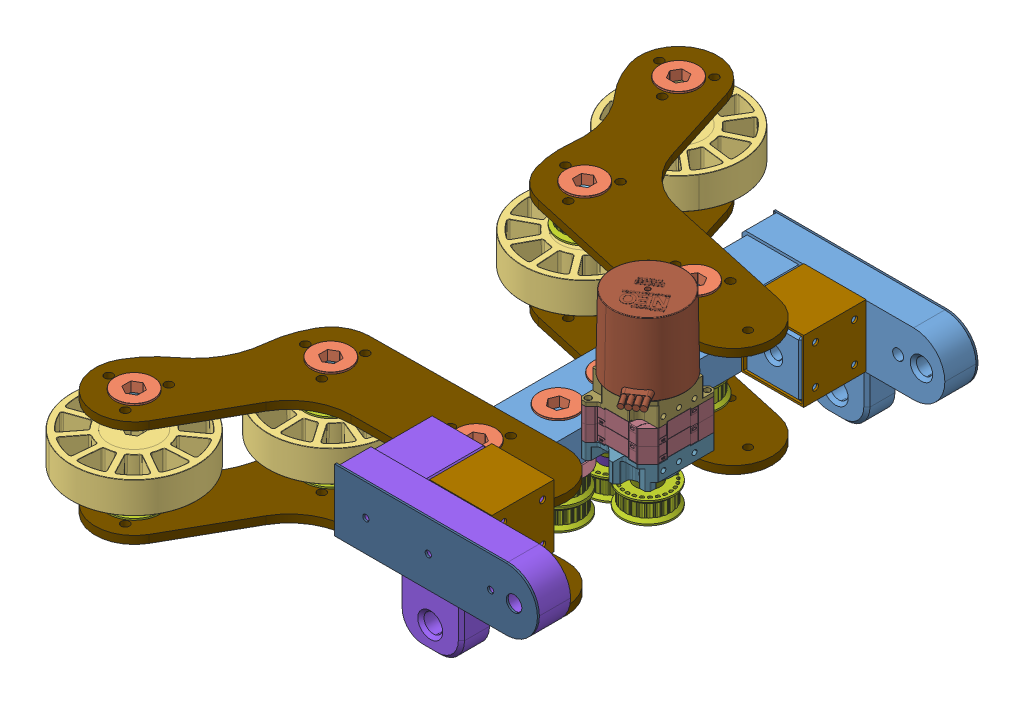
SolidWorks assembly Intake_Claw_2_Wheel_1.0, configuration Default. Lengths in mm.
Overall size (384.98 197.47 557.42).
91 component instances, 20 part files, 331 mates.
Components (placement in the parent):
- Claw_Crossbar-1: Claw_Crossbar [Default] at origin size (50.8 25.4 304.8)
- am-2986 FR8ZZ Hex Bearing.step-1: am-2986 FR8ZZ Hex Bearing.step [Default] at (0 6.2967 88.9) x (-0.023449 0 -0.999725) z (0 1 0) size (31.12 31.12 7.93)
- am-2986 FR8ZZ Hex Bearing.step-3: am-2986 FR8ZZ Hex Bearing.step [Default] at (-175.3573 14.224 192.1035) x (0 0 -1) z (0 1 0) size (31.12 31.12 7.93)
- am-2986 FR8ZZ Hex Bearing.step-5: am-2986 FR8ZZ Hex Bearing.step [Default] at (0 14.224 88.9) x (0 0 -1) z (0 1 0) size (31.12 31.12 7.93)
- am-2986 FR8ZZ Hex Bearing.step-11: am-2986 FR8ZZ Hex Bearing.step [Default] at (-117.4709 14.224 89.8805) x (0 0 -1) z (0 1 0) size (31.12 31.12 7.93)
- Intake_Plate_Assembly-1: Intake_Plate_Assembly [Default] at (-25.3851 110.6877 261.8842) x (0.99204 0 0.125922) z (0.125922 0 -0.99204)
- Intake_Plate_Assembly_2-1: Intake_Plate_Assembly_2 [Default] at (-16.4979 -120.1924 40.8533) x (0.996656 0 -0.081713) z (0.081713 0 0.996656)
- Intake_Plate_Assembly_2-2: Intake_Plate_Assembly_2 [Default] at (-25.364 170.9924 261.8868) x (0.99204 0 0.125922) z (0.125922 0 -0.99204)
- am-3480 4IN 500Hex Bore Compliant Wheel REV2.STEP-1: am-3480 4IN 500Hex Bore Compliant Wheel REV2.STEP [Default] at (-170.665 -13.479 176.0889) x (0.49504 0 -0.86887) z (0 -1 0) size (101.6 101.6 25.4)
- am-3480 4IN 500Hex Bore Compliant Wheel REV2.STEP-3: am-3480 4IN 500Hex Bore Compliant Wheel REV2.STEP [Default] at (-124.708 -13.479 104.9173) x (-0.629902 0 0.776675) z (0 -1 0) size (101.6 101.6 25.4)
- am-3480 4IN 500Hex Bore Compliant Wheel REV2.STEP-4: am-3480 4IN 500Hex Bore Compliant Wheel REV2.STEP [Default] at (-98.6342 4.428 -109.7445) x (0.877194 0 0.480136) z (0 -1 0) size (101.6 101.6 25.4)
- am-3480 4IN 500Hex Bore Compliant Wheel REV2.STEP-6: am-3480 4IN 500Hex Bore Compliant Wheel REV2.STEP [Default] at (-166.0619 4.428 -231.3704) x (-0.851991 0 -0.523557) z (0 -1 0) size (101.6 101.6 25.4)
- am-2986 FR8ZZ Hex Bearing.step-13: am-2986 FR8ZZ Hex Bearing.step [Default] at (0 -6.2967 -22.225) x (-0.368447 0 0.929649) z (0 -1 0) size (31.12 31.12 7.93)
- am-2986 FR8ZZ Hex Bearing.step-14: am-2986 FR8ZZ Hex Bearing.step [Default] at (0 6.2967 -22.225) x (-0.368447 0 0.929649) z (0 1 0) size (31.12 31.12 7.93)
- Claw_Drive_Gear-1: Claw_Drive_Gear [Default] at (0 -26.8478 -22.225) x (0.993752 0 0.111608) z (-0.111608 0 0.993752) size (43.69 9.45 43.69)
- Claw_Drive_Gear-2: Claw_Drive_Gear [Default] at (0 -26.8478 22.225) x (0.964298 0 0.26482) z (-0.26482 0 0.964298) size (43.69 9.45 43.69)
- half_inch_hex_spacer_0.125inch-1: half_inch_hex_spacer_0.125inch [Default] at (0 -17.399 -22.225) x (0.999916 0 -0.012929) z (0.012929 0 0.999916) size (20.32 3.17 20.32)
- half_inch_hex_spacer_0.125inch-2: half_inch_hex_spacer_0.125inch [Default] at (0 -17.399 22.225) x (0.980488 0 0.196577) z (-0.196577 0 0.980488) size (20.32 3.17 20.32)
- am-2986 FR8ZZ Hex Bearing.step-16: am-2986 FR8ZZ Hex Bearing.step [Default] at (0 6.2967 -88.9) x (-0.023449 0 -0.999725) z (0 1 0) size (31.12 31.12 7.93)
- am-2986 FR8ZZ Hex Bearing.step-18: am-2986 FR8ZZ Hex Bearing.step [Default] at (0 -6.2967 -88.9) x (-0.368447 0 0.929649) z (0 -1 0) size (31.12 31.12 7.93)
- am-2986 FR8ZZ Hex Bearing.step-19: am-2986 FR8ZZ Hex Bearing.step [Default] at (0 -6.2967 88.9) x (-0.368447 0 0.929649) z (0 -1 0) size (31.12 31.12 7.93)
- half_inch_hex_spacer_0.1875inch-1: half_inch_hex_spacer_0.1875inch [Default] at (0 14.224 -88.9) size (20.32 4.76 20.32)
- 24_tooth_5mmHTD_timing_belt_pulley_9mm-8: 24_tooth_5mmHTD_timing_belt_pulley_9mm [Default] at (0 -58.5978 22.225) x (0.071014 0 0.997475) z (0 -1 0) size (42.16 42.16 17.78)
- 24_tooth_5mmHTD_timing_belt_pulley_9mm-9: 24_tooth_5mmHTD_timing_belt_pulley_9mm [Default] at (0 -59.8678 -22.225) x (0.476247 0 -0.879312) z (0 -1 0) size (42.16 42.16 17.78)
- 24_tooth_5mmHTD_timing_belt_pulley_9mm-15: 24_tooth_5mmHTD_timing_belt_pulley_9mm [Default] at (-117.4709 -2.921 89.8805) x (0.911482 0 -0.411341) z (0 -1 0) size (42.16 42.16 17.78)
- 24_tooth_5mmHTD_timing_belt_pulley_9mm-16: 24_tooth_5mmHTD_timing_belt_pulley_9mm [Default] at (-114.7265 18.161 -114.1627) x (0.980604 0 0.196) z (0 -1 0) size (42.16 42.16 17.78)
- half_inch_hex_spacer_0.125inch-13: half_inch_hex_spacer_0.125inch [Default] at (-114.7265 11.176 -114.1627) x (0.99974 0 -0.022787) z (0.022787 0 0.99974) size (20.32 3.17 20.32)
- half_inch_hex_spacer_0.125inch-15: half_inch_hex_spacer_0.125inch [Default] at (-150.2116 11.176 -226.1501) x (0.999399 0 -0.034658) z (0.034658 0 0.999399) size (20.32 3.17 20.32)
- half_inch_hex_spacer_0.125inch-16: half_inch_hex_spacer_0.125inch [Default] at (-117.4709 -35.306 89.8805) size (20.32 3.17 20.32)
- half_inch_hex_spacer_0.125inch-18: half_inch_hex_spacer_0.125inch [Default] at (-175.3573 -35.306 192.1035) size (20.32 3.17 20.32)
- Grabber_Spring_Mount_2.0_Right-1: Grabber_Spring_Mount_2.0_Right [Default] at (23.8125 35.8775 101.6) x (-1 0 0) z (0 0 1) size (165.1 95.25 76.2)
- 24_tooth_5mmHTD_timing_belt_pulley_9mm-17: 24_tooth_5mmHTD_timing_belt_pulley_9mm [Default] at (0 -31.369 88.9) x (0.782455 0 -0.622708) z (0 -1 0) size (42.16 42.16 17.78)
- 24_tooth_5mmHTD_timing_belt_pulley_9mm-18: 24_tooth_5mmHTD_timing_belt_pulley_9mm [Default] at (0 -31.369 -88.9) x (0.782455 0 -0.622708) z (0 -1 0) size (42.16 42.16 17.78)
- half_inch_hex_spacer_0.125inch-19: half_inch_hex_spacer_0.125inch [Default] at (0 -17.399 -88.9) size (20.32 3.17 20.32)
- half_inch_hex_spacer_0.125inch-20: half_inch_hex_spacer_0.125inch [Default] at (0 -17.399 88.9) size (20.32 3.17 20.32)
- half_inch_hex_spacer_0.125inch-21: half_inch_hex_spacer_0.125inch [Default] at (-114.7265 -17.399 -114.1627) size (20.32 3.17 20.32)
- half_inch_hex_spacer_0.125inch-23: half_inch_hex_spacer_0.125inch [Default] at (-150.2116 -17.399 -226.1501) size (20.32 3.17 20.32)
- half_inch_hex_spacer_0.125inch-24: half_inch_hex_spacer_0.125inch [Default] at (-175.3573 -38.481 192.1035) size (20.32 3.17 20.32)
- half_inch_hex_spacer_0.125inch-26: half_inch_hex_spacer_0.125inch [Default] at (-117.4709 -38.481 89.8805) size (20.32 3.17 20.32)
- half_inch_hex_spacer_0.125inch-27: half_inch_hex_spacer_0.125inch [Default] at (-117.4709 -59.436 89.8805) size (20.32 3.17 20.32)
- half_inch_hex_spacer_0.125inch-29: half_inch_hex_spacer_0.125inch [Default] at (-175.3573 -59.436 192.1035) size (20.32 3.17 20.32)
- half_inch_hex_spacer_0.125inch-30: half_inch_hex_spacer_0.125inch [Default] at (-114.7265 -38.354 -114.1627) size (20.32 3.17 20.32)
- half_inch_hex_spacer_0.125inch-32: half_inch_hex_spacer_0.125inch [Default] at (-150.2116 -38.354 -226.1501) size (20.32 3.17 20.32)
- 24_tooth_5mmHTD_timing_belt_pulley_9mm-19: 24_tooth_5mmHTD_timing_belt_pulley_9mm [Default] at (-114.7265 -31.369 -114.1627) x (1 0 0) z (0 -1 0) size (42.16 42.16 17.78)
- 24_tooth_5mmHTD_timing_belt_pulley_9mm-21: 24_tooth_5mmHTD_timing_belt_pulley_9mm [Default] at (-150.2116 -31.369 -226.1501) x (1 0 0) z (0 -1 0) size (42.16 42.16 17.78)
- 24_tooth_5mmHTD_timing_belt_pulley_9mm-22: 24_tooth_5mmHTD_timing_belt_pulley_9mm [Default] at (-175.3573 -52.451 192.1035) x (1 0 0) z (0 -1 0) size (42.16 42.16 17.78)
- 24_tooth_5mmHTD_timing_belt_pulley_9mm-24: 24_tooth_5mmHTD_timing_belt_pulley_9mm [Default] at (-117.4709 -52.451 89.8805) x (1 0 0) z (0 -1 0) size (42.16 42.16 17.78)
- half_inch_hex_spacer_0.125inch-33: half_inch_hex_spacer_0.125inch [Default] at (0 -38.354 -88.9) size (20.32 3.17 20.32)
- half_inch_hex_spacer_0.125inch-34: half_inch_hex_spacer_0.125inch [Default] at (0 -38.354 88.9) size (20.32 3.17 20.32)
- Intake_Plate_Assembly-3: Intake_Plate_Assembly [Default] at (-25.3851 78.6304 261.8842) x (0.99204 0 0.125922) z (0.125922 0 -0.99204)
- Intake_Plate_Assembly_2-4: Intake_Plate_Assembly_2 [Default] at (-16.4979 -152.2498 40.8533) x (0.996656 0 -0.081713) z (0.081713 0 0.996656)
- Crossbar_Bracket-1: Crossbar_Bracket [Default] at (76.2 -12.7 -152.4) x (0 1 0) z (0 0 1) size (50.8 50.8 50.8)
- Crossbar_Bracket-2: Crossbar_Bracket [Default] at (76.2 -12.7 101.6) x (0 1 0) z (0 0 1) size (50.8 50.8 50.8)
- Claw_Pivot_Plate-1: Claw_Pivot_Plate [Default] at (-24.765 -13.335 177.8) size (165.1 50.8 1.59)
- Claw_Pivot_Plate-2: Claw_Pivot_Plate [Default] at (-24.765 -13.335 -179.3875) size (165.1 50.8 1.59)
- half_inch_hex_spacer_0.125inch-35: half_inch_hex_spacer_0.125inch [Default] at (-117.4709 11.049 89.8805) size (20.32 3.17 20.32)
- half_inch_hex_spacer_0.125inch-37: half_inch_hex_spacer_0.125inch [Default] at (-175.3573 11.049 192.1035) size (20.32 3.17 20.32)
- half_inch_hex_spacer_0.125inch-38: half_inch_hex_spacer_0.125inch [Default] at (-114.7265 32.131 -114.1627) x (1 0 0.000236) z (-0.000236 0 1) size (20.32 3.17 20.32)
- am-2986 FR8ZZ Hex Bearing.step-20: am-2986 FR8ZZ Hex Bearing.step [Default] at (0 -59.436 88.9) x (1 0 0) z (0 -1 0) size (31.12 31.12 7.93)
- am-2986 FR8ZZ Hex Bearing.step-21: am-2986 FR8ZZ Hex Bearing.step [Default] at (-117.4709 -21.336 89.8805) x (0.820291 0 -0.571946) z (0 -1 0) size (31.12 31.12 7.93)
- am-2986 FR8ZZ Hex Bearing.step-23: am-2986 FR8ZZ Hex Bearing.step [Default] at (-175.3573 -59.436 192.1035) x (1 0 0) z (0 -1 0) size (31.12 31.12 7.93)
- am-2986 FR8ZZ Hex Bearing.step-24: am-2986 FR8ZZ Hex Bearing.step [Default] at (0 -38.354 -88.9) x (1 0 0) z (0 -1 0) size (31.12 31.12 7.93)
- am-2986 FR8ZZ Hex Bearing.step-25: am-2986 FR8ZZ Hex Bearing.step [Default] at (-114.7265 -38.354 -114.1627) x (1 0 0) z (0 -1 0) size (31.12 31.12 7.93)
- am-2986 FR8ZZ Hex Bearing.step-26: am-2986 FR8ZZ Hex Bearing.step [Default] at (-150.2116 -38.354 -226.1501) x (0.059975 0 -0.9982) z (0 -1 0) size (31.12 31.12 7.93)
- am-2986 FR8ZZ Hex Bearing.step-28: am-2986 FR8ZZ Hex Bearing.step [Default] at (0 37.7393 -88.9) x (1 0 0) z (0 1 0) size (31.12 31.12 7.93)
- am-2986 FR8ZZ Hex Bearing.step-31: am-2986 FR8ZZ Hex Bearing.step [Default] at (-150.2116 37.7393 -226.1501) x (1 0 0) z (0 1 0) size (31.12 31.12 7.93)
- am-2986 FR8ZZ Hex Bearing.step-32: am-2986 FR8ZZ Hex Bearing.step [Default] at (0 -6.2967 22.225) x (-0.500268 0 0.865871) z (0 -1 0) size (31.12 31.12 7.93)
- Neo_with_2_Stage_Gearbox-1: Neo_with_2_Stage_Gearbox [Default] at (51.9835 155.825 -0.8874) x (0.196216 0 -0.980561) z (0 -1 0) size (73.48 69 161.54)
  - REV-21-1650-V1.1.step-1: REV-21-1650-V1.1.step [Default] at (-1.1023 -0.9864 105.025) size (68.13 68.01 93.35)
  - REV-21-2106.step-1: REV-21-2106.step [Default] at (-1.1023 -0.9864 114.55) x (0.980561 -0.196216 0) z (0 0 1) size (61.91 50.8 19.05)
  - REV-21-2103.step-1: REV-21-2103.step [Default] at (-1.1023 -0.9864 130.425) x (0.980561 -0.196216 0) z (0 0 1) size (61.91 50.8 16.85)
  - REV-21-2104.step-1: REV-21-2104.step [Default] at (-1.1023 -0.9864 159) x (0 0 1) z (-0.980561 0.196216 0) size (23.2 50.8 61.92)
  - REV-21-2103.step-2: REV-21-2103.step [Default] at (-1.1023 -0.9864 143.125) x (0.980561 -0.196216 0) z (0 0 1) size (61.91 50.8 16.85)
  - motor_drive_shaft-1: motor_drive_shaft [Default] at (-1.1023 -0.9864 157.4125) x (0.381586 -0.924333 0) z (0 0 1) size (14.66 12.7 50.8)
- half_inch_hex_spacer_0.125inch-40: half_inch_hex_spacer_0.125inch [Default] at (0 -49.4563 -88.9) x (0.980488 0 0.196577) z (-0.196577 0 0.980488) size (20.32 3.17 20.32)
- half_inch_hex_spacer_0.125inch-41: half_inch_hex_spacer_0.125inch [Default] at (0 -70.5383 88.9) x (0.980488 0 0.196577) z (-0.196577 0 0.980488) size (20.32 3.17 20.32)
- 24_tooth_5mmHTD_timing_belt_pulley_9mm-25: 24_tooth_5mmHTD_timing_belt_pulley_9mm [Default] at (0 -63.4263 -88.9) x (1 0 0) z (0 -1 0) size (42.16 42.16 17.78)
- 24_tooth_5mmHTD_timing_belt_pulley_9mm-26: 24_tooth_5mmHTD_timing_belt_pulley_9mm [Default] at (0 -84.5083 88.9) x (1 0 0) z (0 -1 0) size (42.16 42.16 17.78)
- half_inch_hex_spacer_0.5inch-1: half_inch_hex_spacer_0.5inch [Default] at (0 -39.5478 -22.225) size (20.32 12.7 20.32)
- half_inch_hex_spacer_0.5inch-2: half_inch_hex_spacer_0.5inch [Default] at (50.8 -25.4 0) size (20.32 12.7 20.32)
- half_inch_hex_spacer_0.25inch-1: half_inch_hex_spacer_0.25inch [Default] at (0 -45.8978 -22.225) size (20.32 6.35 20.32)
- am-4700_syc Cone-1: am-4700_syc Cone [Default] at (-103.1993 110.9219 -0.8914) x (0.984784 0.17378 0) z (0 0 -1) size (212.72 325.44 212.72) (hidden)
- Claw_Intake_Plate_2_Wheel-1: Claw_Intake_Plate_2_Wheel [Default] at (0 -65.8393 88.9) x (-0.008346 0 -0.999965) z (0.999965 0 -0.008346) size (165.24 6.35 280.99)
- Claw_Intake_Plate_2_Wheel-2: Claw_Intake_Plate_2_Wheel [Default] at (0 14.2773 88.9) x (-0.008346 0 -0.999965) z (0.999965 0 -0.008346) size (165.24 6.35 280.99)
- Claw_Intake_Plate_2_Wheel-3: Claw_Intake_Plate_2_Wheel [Default] at (0 44.1427 -88.9) x (-0.215048 0 0.976604) z (0.976604 0 0.215048) size (165.24 6.35 280.99)
- Claw_Intake_Plate_2_Wheel-4: Claw_Intake_Plate_2_Wheel [Default] at (0 -38.4073 -88.9) x (-0.215048 0 0.976604) z (0.976604 0 0.215048) size (165.24 6.35 280.99)
- am-2986 FR8ZZ Hex Bearing.step-33: am-2986 FR8ZZ Hex Bearing.step [Default] at (-114.7265 37.7393 -114.1627) x (0 0 -1) z (0 1 0) size (31.12 31.12 7.93)
- am-2986 FR8ZZ Hex Bearing.step-34: am-2986 FR8ZZ Hex Bearing.step [Default] at (0 6.2967 22.225) x (-0.368447 0 0.929649) z (0 1 0) size (31.12 31.12 7.93)
- 24_tooth_5mmHTD_timing_belt_pulley_9mm-27: 24_tooth_5mmHTD_timing_belt_pulley_9mm [Default] at (50.8 -39.37 0) x (0.071014 0 0.997475) z (0 -1 0) size (42.16 42.16 17.78)
- 24_tooth_5mmHTD_timing_belt_pulley_9mm-28: 24_tooth_5mmHTD_timing_belt_pulley_9mm [Default] at (0 -40.8178 22.225) x (0.071014 0 0.997475) z (0 -1 0) size (42.16 42.16 17.78)
- Grabber_Spring_Mount_2.0_Left-1: Grabber_Spring_Mount_2.0_Left [Default] at (23.8125 -11.7475 -101.6) x (-1 0 0) z (0 0 -1) size (165.1 95.25 76.2)
Mates (geometry in assembly coordinates):
- Concentric2: concentric aligned: circle of Claw_Crossbar-1; circle of Claw_Intake_Plates-3
- Concentric5: concentric aligned: circle of Claw_Crossbar-1; circle of am-2986 FR8ZZ Hex Bearing.step-1
- Coincident11: coincident anti-aligned: plane of Claw_Crossbar-1 through (-25.4 12.7 152.4) normal (0 1 0); plane of am-2986 FR8ZZ Hex Bearing.step-1 through (-0.3276 12.7 74.9338) normal (0 -1 0)
- Concentric6: concentric anti-aligned: cylinder of Claw_Intake_Plates-3; cylinder of am-2986 FR8ZZ Hex Bearing.step-5 through (0 22.1513 88.9) axis (0 -1 0) radius 15.5575
- Coincident12: coincident anti-aligned: plane of Claw_Intake_Plates-3 through (-239.4221 58.7273 343.7898) normal (0 1 0); plane of am-2986 FR8ZZ Hex Bearing.step-5 through (0 20.6273 74.93) normal (0 -1 0)
- Concentric7: concentric aligned: circle of Claw_Intake_Plates-3; circle of am-2986 FR8ZZ Hex Bearing.step-11
- Coincident13: coincident anti-aligned: plane of Claw_Intake_Plates-3 through (-239.4221 58.7273 343.7898) normal (0 1 0); plane of am-2986 FR8ZZ Hex Bearing.step-11 through (-117.4709 20.6273 75.9105) normal (0 -1 0)
- Concentric9: concentric aligned: circle of Claw_Intake_Plates-3; circle of am-2986 FR8ZZ Hex Bearing.step-3
- Coincident15: coincident anti-aligned: plane of Claw_Intake_Plates-3 through (-239.4221 58.7273 343.7898) normal (0 1 0); plane of am-2986 FR8ZZ Hex Bearing.step-3 through (-175.3573 20.6273 178.1335) normal (0 -1 0)
- Concentric10: concentric anti-aligned: circle of Claw_Crossbar-1; circle of Intake_Plate_Assembly-1/am-2986 FR8ZZ Hex Bearing.step-5
- Concentric11: concentric aligned: circle of Claw_Crossbar-1; circle of Intake_Plate_Assembly_2-1/Claw_Intake_Plates-3
- Concentric12: concentric anti-aligned: circle of Claw_Crossbar-1; circle of Intake_Plate_Assembly_2-2/Claw_Intake_Plates-3
- Parallel3: parallel aligned: plane of Intake_Plate_Assembly-1/Claw_Intake_Plates-3 through (77.0074 -7.9273 33.08) normal (0.025971 0 -0.999663); plane of Intake_Plate_Assembly_2-2/Claw_Intake_Plates-3 through (77.0074 52.3773 33.08) normal (0.025971 0 -0.999663)
- Parallel4: parallel aligned: plane of Claw_Intake_Plates-3 through (76.2901 58.7273 272.9054) normal (0.002844 0 0.999996); plane of Intake_Plate_Assembly_2-1/Claw_Intake_Plates-3 through (75.6047 -1.5773 273.9833) normal (-0.018478 0 0.999829)
- Concentric17: concentric anti-aligned: circle of Intake_Plate_Assembly_2-1/am-2986 FR8ZZ Hex Bearing.step-18; circle of am-3480 4IN 500Hex Bore Compliant Wheel REV2.STEP-1
- Concentric18: concentric anti-aligned: circle of Intake_Plate_Assembly_2-1/am-2986 FR8ZZ Hex Bearing.step-17; circle of am-3480 4IN 500Hex Bore Compliant Wheel REV2.STEP-2
- Concentric20: concentric anti-aligned: circle of Intake_Plate_Assembly-1/am-2986 FR8ZZ Hex Bearing.step-12; circle of am-3480 4IN 500Hex Bore Compliant Wheel REV2.STEP-5
- Concentric21: concentric aligned: circle of Intake_Plate_Assembly-1/am-2986 FR8ZZ Hex Bearing.step-11; circle of am-3480 4IN 500Hex Bore Compliant Wheel REV2.STEP-4
- Concentric22: concentric anti-aligned: circle of Intake_Plate_Assembly-1/am-2986 FR8ZZ Hex Bearing.step-3; circle of am-3480 4IN 500Hex Bore Compliant Wheel REV2.STEP-6
- Coincident21: coincident aligned: plane of am-3480 4IN 500Hex Bore Compliant Wheel REV2.STEP-5 through (-180.9613 5.969 86.3864) normal (0 -1 0); plane of am-3480 4IN 500Hex Bore Compliant Wheel REV2.STEP-6 through (-139.4727 -14.224 -243.6257) normal (0 -1 0)
- Coincident22: coincident aligned: plane of am-3480 4IN 500Hex Bore Compliant Wheel REV2.STEP-4 through (-124.5748 -14.224 -96.1701) normal (0 -1 0); plane of am-3480 4IN 500Hex Bore Compliant Wheel REV2.STEP-5 through (-180.9613 5.969 86.3864) normal (0 -1 0)
- Coincident23: coincident aligned: plane of am-3480 4IN 500Hex Bore Compliant Wheel REV2.STEP-2 through (-168.4561 5.969 258.1356) normal (0 -1 0); plane of am-3480 4IN 500Hex Bore Compliant Wheel REV2.STEP-4 through (-124.5748 -14.224 -96.1701) normal (0 -1 0)
- Coincident24: coincident aligned: plane of am-3480 4IN 500Hex Bore Compliant Wheel REV2.STEP-1 through (-157.5354 -32.131 202.2575) normal (0 -1 0); plane of am-3480 4IN 500Hex Bore Compliant Wheel REV2.STEP-2 through (-168.4561 5.969 258.1356) normal (0 -1 0)
- Coincident25: coincident aligned: plane of am-3480 4IN 500Hex Bore Compliant Wheel REV2.STEP-1 through (-157.5354 -32.131 202.2575) normal (0 -1 0); plane of am-3480 4IN 500Hex Bore Compliant Wheel REV2.STEP-3 through (-133.4017 -32.131 76.9602) normal (0 -1 0)
- Concentric23: concentric anti-aligned: circle of Intake_Plate_Assembly_2-1/am-2986 FR8ZZ Hex Bearing.step-11; circle of am-3480 4IN 500Hex Bore Compliant Wheel REV2.STEP-3
- Coincident26: coincident aligned: plane of Intake_Plate_Assembly-1/Claw_Intake_Plates-3 through (-236.9809 -7.9273 -45.0872) normal (0 -1 0); plane of Intake_Plate_Assembly_2-1/Claw_Intake_Plates-3 through (-241.5471 -7.9273 338.1202) normal (0 -1 0)
- Coincident27: coincident aligned: plane of Claw_Intake_Plates-3 through (-239.4221 52.3773 343.7898) normal (0 -1 0); plane of Intake_Plate_Assembly_2-2/Claw_Intake_Plates-3 through (-236.9809 52.3773 -45.0872) normal (0 -1 0)
- Parallel6: parallel aligned: plane of Claw_Crossbar-1 through (25.4 -12.7 152.4) normal (1 0 0); plane of REV-21-2103.step-1 through (50.8 -18.7019 200.025) normal (1 0 0)
- Concentric26: concentric anti-aligned: circle of Claw_Crossbar-1; circle of am-2986 FR8ZZ Hex Bearing.step-13
- Coincident30: coincident anti-aligned: plane of Claw_Crossbar-1 through (-25.4 -12.7 152.4) normal (0 -1 0); plane of am-2986 FR8ZZ Hex Bearing.step-13 through (-5.1472 -12.7 -9.2378) normal (0 1 0)
- Concentric27: concentric anti-aligned: circle of Claw_Crossbar-1; circle of am-2986 FR8ZZ Hex Bearing.step-14
- Concentric28: concentric anti-aligned: circle of Claw_Crossbar-1; circle of am-2986 FR8ZZ Hex Bearing.step-15
- Coincident31: coincident anti-aligned: plane of Claw_Crossbar-1 through (-25.4 12.7 152.4) normal (0 1 0); plane of am-2986 FR8ZZ Hex Bearing.step-15 through (20.2528 50.8 187.6122) normal (0 -1 0)
- Coincident32: coincident anti-aligned: plane of Claw_Crossbar-1 through (-25.4 12.7 152.4) normal (0 1 0); plane of am-2986 FR8ZZ Hex Bearing.step-14 through (-5.1472 12.7 -9.2378) normal (0 -1 0)
- Concentric29: concentric aligned: circle of am-2986 FR8ZZ Hex Bearing.step-14; circle of Claw_Drive_Gear-1
- Concentric30: concentric anti-aligned: circle of am-2986 FR8ZZ Hex Bearing.step-15; circle of Claw_Drive_Gear-2
- Concentric31: concentric anti-aligned: circle of am-2986 FR8ZZ Hex Bearing.step-14; circle of half_inch_hex_spacer_0.125inch-1
- Concentric32: concentric anti-aligned: circle of am-2986 FR8ZZ Hex Bearing.step-15; circle of half_inch_hex_spacer_0.125inch-2
- Coincident37: coincident anti-aligned: plane of Claw_Drive_Gear-1 through (0 -17.399 -22.225) normal (0 1 0); plane of half_inch_hex_spacer_0.125inch-3 through (25.4 64.9478 130.556) normal (0 -1 0)
- Concentric33: concentric aligned: circle of Claw_Drive_Gear-1; circle of half_inch_hex_spacer_0.125inch-3
- Coincident38: coincident anti-aligned: plane of Claw_Drive_Gear-2 through (0 -17.399 22.225) normal (0 1 0); plane of half_inch_hex_spacer_0.125inch-4 through (25.4 64.9478 174.244) normal (0 -1 0)
- Concentric34: concentric aligned: circle of Claw_Drive_Gear-2; circle of half_inch_hex_spacer_0.125inch-4
- Coincident39: coincident anti-aligned: plane of Claw_Crossbar-1 through (-25.4 12.7 152.4) normal (0 1 0); plane of am-2986 FR8ZZ Hex Bearing.step-16 through (-0.3276 12.7 -102.8662) normal (0 -1 0)
- Concentric35: concentric anti-aligned: circle of Claw_Crossbar-1; circle of am-2986 FR8ZZ Hex Bearing.step-16
- Coincident40: coincident anti-aligned: plane of Claw_Crossbar-1 through (-25.4 -12.7 152.4) normal (0 -1 0); plane of am-2986 FR8ZZ Hex Bearing.step-18 through (-5.1472 -12.7 -75.9128) normal (0 1 0)
- Coincident41: coincident anti-aligned: plane of Claw_Crossbar-1 through (-25.4 -12.7 152.4) normal (0 -1 0); plane of am-2986 FR8ZZ Hex Bearing.step-19 through (-5.1472 -12.7 101.8872) normal (0 1 0)
- Concentric36: concentric anti-aligned: circle of Claw_Crossbar-1; circle of am-2986 FR8ZZ Hex Bearing.step-19
- Concentric37: concentric anti-aligned: circle of Claw_Crossbar-1; circle of am-2986 FR8ZZ Hex Bearing.step-18
- Coincident42: coincident anti-aligned: plane of Intake_Plate_Assembly_2-1/am-2986 FR8ZZ Hex Bearing.step-16 through (25.4 -1.524 241.3) normal (0 1 0); plane of am-2986 FR8ZZ Hex Bearing.step-19 through (-5.7321 -14.224 103.363) normal (0 -1 0)
- Coincident43: coincident anti-aligned: plane of am-2986 FR8ZZ Hex Bearing.step-1 through (-0.3648 14.224 73.3468) normal (0 1 0); plane of am-2986 FR8ZZ Hex Bearing.step-5 through (0 14.224 88.9) normal (0 -1 0)
- Coincident45: coincident anti-aligned: plane of Claw_Drive_Gear-1 through (0 -17.399 -22.225) normal (0 1 0); plane of 18_tooth_5mmHTD_timing_belt_pulley_9mm-1 through (25.4 64.9478 130.556) normal (0 -1 0)
- Concentric39: concentric aligned: circle of Claw_Drive_Gear-1; circle of 18_tooth_5mmHTD_timing_belt_pulley_9mm-1
- Parallel7: parallel anti-aligned: plane of Claw_Drive_Gear-2 through (0 -26.8478 22.225) normal (0 -1 0); plane of half_inch_hex_spacer_0.125inch-4 through (25.4 68.1228 174.244) normal (0 1 0)
- Coincident48: coincident anti-aligned: plane of 18_tooth_5mmHTD_timing_belt_pulley_9mm-1 through (25.4 82.7278 130.556) normal (0 1 0); plane of half_inch_hex_collar-2 through (25.4 82.7278 130.556) normal (0 -1 0)
- Concentric42: concentric aligned: circle of 18_tooth_5mmHTD_timing_belt_pulley_9mm-1; circle of half_inch_hex_collar-2
- Coincident50: coincident anti-aligned: plane of am-2986 FR8ZZ Hex Bearing.step-5 through (0 22.1513 73.3425) normal (0 1 0); plane of half_inch_hex_spacer_0.125inch-5 through (25.4 60.2513 241.3) normal (0 -1 0)
- Coincident51: coincident aligned: plane of Intake_Plate_Assembly_2-2/am-2986 FR8ZZ Hex Bearing.step-16 through (23.441 60.2513 78.9337) normal (0 1 0); circle of half_inch_hex_spacer_0.125inch-6
- Concentric43: concentric aligned: circle of Intake_Plate_Assembly_2-2/am-2986 FR8ZZ Hex Bearing.step-16; circle of half_inch_hex_spacer_0.125inch-6
- Concentric44: concentric aligned: circle of am-2986 FR8ZZ Hex Bearing.step-5; circle of half_inch_hex_spacer_0.125inch-5
- Coincident52: coincident anti-aligned: plane of am-2986 FR8ZZ Hex Bearing.step-5 through (0 22.1513 73.3425) normal (0 1 0); plane of half_inch_hex_spacer_0.1875inch-2 through (25.4 60.2513 241.3) normal (0 -1 0)
- Concentric45: concentric aligned: circle of am-2986 FR8ZZ Hex Bearing.step-5; circle of half_inch_hex_spacer_0.1875inch-2
- Coincident54: coincident anti-aligned: plane of Intake_Plate_Assembly_2-2/am-2986 FR8ZZ Hex Bearing.step-16 through (23.441 60.2513 78.9337) normal (0 1 0); plane of half_inch_hex_spacer_0.1875inch-1 through (0 14.224 -88.9) normal (0 -1 0)
- Concentric47: concentric aligned: circle of Intake_Plate_Assembly_2-2/am-2986 FR8ZZ Hex Bearing.step-16; circle of half_inch_hex_spacer_0.1875inch-1
- Concentric55: concentric aligned: circle of am-2986 FR8ZZ Hex Bearing.step-3; circle of 24_tooth_5mmHTD_timing_belt_pulley_9mm-2
- Concentric57: concentric aligned: circle of am-2986 FR8ZZ Hex Bearing.step-11; circle of 24_tooth_5mmHTD_timing_belt_pulley_9mm-4
- Concentric58: concentric aligned: circle of Intake_Plate_Assembly_2-2/am-2986 FR8ZZ Hex Bearing.step-18; circle of 24_tooth_5mmHTD_timing_belt_pulley_9mm-6
- Concentric59: concentric aligned: circle of Intake_Plate_Assembly_2-2/am-2986 FR8ZZ Hex Bearing.step-17; circle of 24_tooth_5mmHTD_timing_belt_pulley_9mm-5
- Concentric60: concentric anti-aligned: circle of Intake_Plate_Assembly_2-2/am-2986 FR8ZZ Hex Bearing.step-11; circle of 24_tooth_5mmHTD_timing_belt_pulley_9mm-1
- Coincident58: coincident anti-aligned: plane of half_inch_hex_spacer_0.1875inch-2 through (25.4 65.0138 241.3) normal (0 1 0); plane of 24_tooth_5mmHTD_timing_belt_pulley_9mm-7 through (25.4 65.0138 241.3) normal (0 -1 0)
- Concentric61: concentric anti-aligned: circle of half_inch_hex_spacer_0.1875inch-2; circle of 24_tooth_5mmHTD_timing_belt_pulley_9mm-7
- Concentric62: concentric anti-aligned: circle of Claw_Drive_Gear-1; circle of 24_tooth_5mmHTD_timing_belt_pulley_9mm-9
- Concentric63: concentric anti-aligned: circle of Claw_Drive_Gear-2; circle of 24_tooth_5mmHTD_timing_belt_pulley_9mm-8
- Coincident61: coincident anti-aligned: plane of half_inch_hex_spacer_0.1875inch-1 through (0 18.9865 -88.9) normal (0 1 0); plane of 24_tooth_5mmHTD_timing_belt_pulley_9mm-10 through (25.4 57.0865 63.5) normal (0 -1 0)
- Concentric64: concentric anti-aligned: circle of half_inch_hex_spacer_0.1875inch-1; circle of 24_tooth_5mmHTD_timing_belt_pulley_9mm-10
- Coincident62: coincident aligned: circle of 24_tooth_5mmHTD_timing_belt_pulley_9mm-4; circle of 24_tooth_5mmHTD_timing_belt_pulley_9mm-11
- Concentric65: concentric anti-aligned: circle of Intake_Plate_Assembly_2-2/am-2986 FR8ZZ Hex Bearing.step-17; circle of 24_tooth_5mmHTD_timing_belt_pulley_9mm-5
- Concentric66: concentric anti-aligned: circle of Intake_Plate_Assembly_2-2/am-2986 FR8ZZ Hex Bearing.step-17; circle of 24_tooth_5mmHTD_timing_belt_pulley_9mm-13
- Concentric68: concentric anti-aligned: circle of Intake_Plate_Assembly_2-2/am-2986 FR8ZZ Hex Bearing.step-11; circle of 24_tooth_5mmHTD_timing_belt_pulley_9mm-16
- Concentric69: concentric anti-aligned: circle of am-2986 FR8ZZ Hex Bearing.step-11; circle of 24_tooth_5mmHTD_timing_belt_pulley_9mm-15
- Coincident67: coincident anti-aligned: plane of am-3480 4IN 500Hex Bore Compliant Wheel REV2.STEP-3 through (-119.4437 -6.731 88.2805) normal (0 1 0); plane of 24_tooth_5mmHTD_timing_belt_pulley_9mm-15 through (-117.4709 -6.731 89.8805) normal (0 -1 0)
- Coincident68: coincident anti-aligned: plane of am-3480 4IN 500Hex Bore Compliant Wheel REV2.STEP-5 through (-180.9613 31.369 68.4149) normal (0 1 0); plane of 24_tooth_5mmHTD_timing_belt_pulley_9mm-13 through (-180.9613 31.369 65.8749) normal (0 -1 0)
- Coincident69: coincident anti-aligned: plane of am-3480 4IN 500Hex Bore Compliant Wheel REV2.STEP-2 through (-179.424 31.369 243.899) normal (0 1 0); plane of 24_tooth_5mmHTD_timing_belt_pulley_9mm-3 through (-180.9742 31.369 241.8869) normal (0 -1 0)
- Coincident73: coincident anti-aligned: plane of am-3480 4IN 500Hex Bore Compliant Wheel REV2.STEP-5 through (-180.9613 5.969 86.3864) normal (0 -1 0); plane of half_inch_hex_spacer_0.125inch-14 through (-180.9613 5.969 65.8749) normal (0 1 0)
- Concentric71: concentric aligned: circle of am-3480 4IN 500Hex Bore Compliant Wheel REV2.STEP-5; circle of half_inch_hex_spacer_0.125inch-14
- Coincident75: coincident anti-aligned: plane of am-3480 4IN 500Hex Bore Compliant Wheel REV2.STEP-3 through (-133.4017 -32.131 76.9602) normal (0 -1 0); plane of half_inch_hex_spacer_0.125inch-16 through (-117.4709 -32.131 89.8805) normal (0 1 0)
- Concentric73: concentric aligned: circle of am-3480 4IN 500Hex Bore Compliant Wheel REV2.STEP-3; circle of half_inch_hex_spacer_0.125inch-16
- Coincident76: coincident anti-aligned: plane of am-3480 4IN 500Hex Bore Compliant Wheel REV2.STEP-2 through (-168.4561 5.969 258.1356) normal (0 -1 0); plane of half_inch_hex_spacer_0.125inch-17 through (-180.9742 5.969 241.8869) normal (0 1 0)
- Concentric74: concentric aligned: circle of am-3480 4IN 500Hex Bore Compliant Wheel REV2.STEP-2; circle of half_inch_hex_spacer_0.125inch-17
- Coincident77: coincident anti-aligned: plane of am-3480 4IN 500Hex Bore Compliant Wheel REV2.STEP-1 through (-157.5354 -32.131 202.2575) normal (0 -1 0); plane of half_inch_hex_spacer_0.125inch-18 through (-175.3573 -32.131 192.1035) normal (0 1 0)
- Concentric75: concentric aligned: cylinder of am-3480 4IN 500Hex Bore Compliant Wheel REV2.STEP-1 through (-175.3573 -61.9272 192.1035) axis (0 1 0) radius 50.8; circle of half_inch_hex_spacer_0.125inch-18
- Coincident78: coincident anti-aligned: plane of am-2986 FR8ZZ Hex Bearing.step-3 through (-175.3573 22.1513 176.546) normal (0 1 0); plane of half_inch_hex_spacer_0.125inch-9 through (-230.4157 60.2513 364.5609) normal (0 -1 0)
- Concentric76: concentric anti-aligned: circle of am-2986 FR8ZZ Hex Bearing.step-3; circle of half_inch_hex_spacer_0.125inch-9
- Coincident80: coincident anti-aligned: plane of am-2986 FR8ZZ Hex Bearing.step-11 through (-117.4709 22.1513 74.323) normal (0 1 0); plane of half_inch_hex_spacer_0.125inch-12 through (-63.197 60.2513 248.6341) normal (0 -1 0)
- Concentric78: concentric anti-aligned: circle of am-2986 FR8ZZ Hex Bearing.step-11; circle of half_inch_hex_spacer_0.125inch-12
- Coincident81: coincident anti-aligned: plane of 24_tooth_5mmHTD_timing_belt_pulley_9mm-4 through (-63.197 63.4263 248.6341) normal (0 -1 0); circle of half_inch_hex_spacer_0.125inch-12
- Coincident83: coincident anti-aligned: plane of 24_tooth_5mmHTD_timing_belt_pulley_9mm-2 through (-230.4157 63.4263 364.5609) normal (0 -1 0); plane of half_inch_hex_spacer_0.125inch-9 through (-230.4157 63.4263 364.5609) normal (0 1 0)
- Coincident84: coincident anti-aligned: plane of 24_tooth_5mmHTD_timing_belt_pulley_9mm-14 through (-180.2715 63.4263 258.3256) normal (0 -1 0); plane of half_inch_hex_spacer_0.125inch-10 through (-180.2715 63.4263 258.3256) normal (0 1 0)
- Coincident85: coincident anti-aligned: plane of Intake_Plate_Assembly_2-2/am-2986 FR8ZZ Hex Bearing.step-11 through (-65.429 60.2513 76.6249) normal (0 1 0); plane of half_inch_hex_spacer_0.125inch-11 through (-63.3778 60.2513 58.8404) normal (0 -1 0)
- Concentric79: concentric anti-aligned: circle of Intake_Plate_Assembly_2-2/am-2986 FR8ZZ Hex Bearing.step-11; circle of half_inch_hex_spacer_0.125inch-11
- Coincident86: coincident anti-aligned: plane of 24_tooth_5mmHTD_timing_belt_pulley_9mm-12 through (-63.3778 63.4263 58.8404) normal (0 -1 0); plane of half_inch_hex_spacer_0.125inch-11 through (-63.3778 63.4263 58.8404) normal (0 1 0)
- Coincident87: coincident anti-aligned: plane of Intake_Plate_Assembly_2-2/am-2986 FR8ZZ Hex Bearing.step-18 through (-238.9399 60.2513 -29.6536) normal (0 1 0); plane of half_inch_hex_spacer_0.125inch-8 through (-234.0156 60.2513 -51.9922) normal (0 -1 0)
- Concentric80: concentric anti-aligned: circle of Intake_Plate_Assembly_2-2/am-2986 FR8ZZ Hex Bearing.step-18; circle of half_inch_hex_spacer_0.125inch-8
- Coincident88: coincident anti-aligned: plane of 24_tooth_5mmHTD_timing_belt_pulley_9mm-6 through (-234.0156 63.4263 -51.9922) normal (0 -1 0); plane of half_inch_hex_spacer_0.125inch-8 through (-234.0156 63.4263 -51.9922) normal (0 1 0)
- Coincident89: coincident anti-aligned: plane of Intake_Plate_Assembly_2-2/am-2986 FR8ZZ Hex Bearing.step-17 through (-182.8644 60.2513 73.5739) normal (0 1 0); plane of half_inch_hex_spacer_0.125inch-7 through (-180.6913 60.2513 52.683) normal (0 -1 0)
- Concentric81: concentric aligned: circle of Intake_Plate_Assembly_2-2/am-2986 FR8ZZ Hex Bearing.step-17; circle of half_inch_hex_spacer_0.125inch-7
- Coincident90: coincident anti-aligned: plane of 24_tooth_5mmHTD_timing_belt_pulley_9mm-5 through (-180.6913 63.4263 52.683) normal (0 -1 0); plane of half_inch_hex_spacer_0.125inch-7 through (-180.6913 63.4263 52.683) normal (0 1 0)
- Coincident95: coincident anti-aligned: plane of Claw_Crossbar-1 through (0 0 -152.4) normal (0 0 -1); plane of Grabber_Spring_Mount_2.0-2 through (49.3395 1.5875 0) normal (0 0 1)
- Coincident101: coincident anti-aligned: plane of Intake_Plate_Assembly-1/am-2986 FR8ZZ Hex Bearing.step-5 through (23.441 -9.4513 78.9337) normal (0 -1 0); plane of half_inch_hex_spacer_0.125inch-19 through (0 -14.224 -88.9) normal (0 1 0)
- Concentric82: concentric anti-aligned: circle of Intake_Plate_Assembly-1/am-2986 FR8ZZ Hex Bearing.step-5; circle of half_inch_hex_spacer_0.125inch-19
- Coincident102: coincident anti-aligned: plane of 24_tooth_5mmHTD_timing_belt_pulley_9mm-18 through (0 -17.399 -88.9) normal (0 1 0); plane of half_inch_hex_spacer_0.125inch-19 through (0 -17.399 -88.9) normal (0 -1 0)
- Concentric83: concentric aligned: cylinder of 24_tooth_5mmHTD_timing_belt_pulley_9mm-18 through (0 -35.179 -88.9) axis (0 1 0) radius 21.082; circle of half_inch_hex_spacer_0.125inch-19
- Coincident103: coincident anti-aligned: plane of Intake_Plate_Assembly_2-1/am-2986 FR8ZZ Hex Bearing.step-16 through (24.1288 -9.4513 225.7945) normal (0 -1 0); plane of half_inch_hex_spacer_0.125inch-20 through (0 -14.224 88.9) normal (0 1 0)
- Concentric84: concentric aligned: circle of Intake_Plate_Assembly_2-1/am-2986 FR8ZZ Hex Bearing.step-16; circle of half_inch_hex_spacer_0.125inch-20
- Coincident104: coincident anti-aligned: plane of 24_tooth_5mmHTD_timing_belt_pulley_9mm-17 through (0 -17.399 88.9) normal (0 1 0); plane of half_inch_hex_spacer_0.125inch-20 through (0 -17.399 88.9) normal (0 -1 0)
- Concentric85: concentric anti-aligned: circle of 24_tooth_5mmHTD_timing_belt_pulley_9mm-17; circle of half_inch_hex_spacer_0.125inch-20
- Coincident105: coincident anti-aligned: plane of Intake_Plate_Assembly-1/am-2986 FR8ZZ Hex Bearing.step-11 through (-65.429 -9.4513 76.6249) normal (0 -1 0); plane of half_inch_hex_spacer_0.125inch-21 through (-114.7265 -14.224 -114.1627) normal (0 1 0)
- Concentric86: concentric anti-aligned: circle of Intake_Plate_Assembly-1/am-2986 FR8ZZ Hex Bearing.step-11; circle of half_inch_hex_spacer_0.125inch-21
- Coincident106: coincident anti-aligned: plane of half_inch_hex_spacer_0.125inch-21 through (-114.7265 -17.399 -114.1627) normal (0 -1 0); plane of 24_tooth_5mmHTD_timing_belt_pulley_9mm-19 through (-114.7265 -17.399 -114.1627) normal (0 1 0)
- Concentric87: concentric anti-aligned: circle of half_inch_hex_spacer_0.125inch-21; circle of 24_tooth_5mmHTD_timing_belt_pulley_9mm-19
- Coincident107: coincident anti-aligned: plane of half_inch_hex_spacer_0.125inch-30 through (-114.7265 -35.179 -114.1627) normal (0 1 0); plane of 24_tooth_5mmHTD_timing_belt_pulley_9mm-19 through (-114.7265 -35.179 -114.1627) normal (0 -1 0)
- Concentric88: concentric anti-aligned: circle of half_inch_hex_spacer_0.125inch-30; circle of 24_tooth_5mmHTD_timing_belt_pulley_9mm-19
- Coincident108: coincident anti-aligned: plane of Intake_Plate_Assembly-1/am-2986 FR8ZZ Hex Bearing.step-12 through (-182.8644 -9.4513 73.5739) normal (0 -1 0); plane of half_inch_hex_spacer_0.125inch-22 through (-180.9613 2.794 65.8749) normal (0 1 0)
- Concentric89: concentric anti-aligned: circle of Intake_Plate_Assembly-1/am-2986 FR8ZZ Hex Bearing.step-12; circle of half_inch_hex_spacer_0.125inch-22
